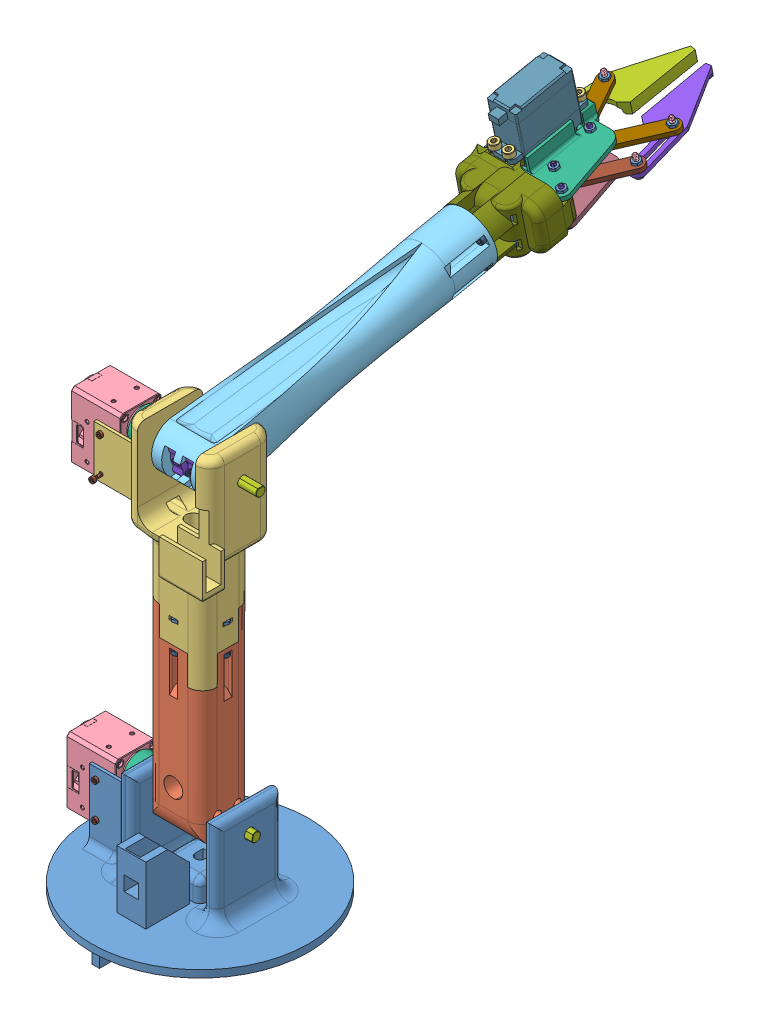
SolidWorks assembly Arm, configuration Défaut. Lengths in mm.
Overall size (155 388.61 426.09).
111 component instances, 29 part files, 108 mates.
Components (placement in the parent):
- arm_base-1: arm_base [Défaut] at (-76.3133 -23.0918 0) size (150 75 150)
- inferior_segment_1-1: inferior_segment_1 [Défaut] at (-77.3133 36.0082 -0.0041) x (1 0 0) z (0 0.001126 0.999999) size (42.86 137.5 35)
- superior_segment_1-1: superior_segment_1 [Défaut] at (-77.1133 116.0083 0.1059) x (1 0 0) z (0 0.001126 0.999999) size (91 145 55)
- XM430-W350-1: XM430-W350 [Default] at (-137.3133 32.4082 0) x (0 0 -1) z (1 0 0) size (28.5 46.5 42.4)
- segment_2-1: segment_2 [Default] at (-77.1133 240.5082 -0.0343) x (-1 0 0) z (0 0.200343 -0.979726) size (38.54 37.14 206.68)
- gripper-1: gripper [Predeterminado] at (-76.3096 293.9805 -248.1519) x (-1 0 0) z (0 -0.200343 0.979726) size (83.16 69.34 163.57)
  - superior_gripper_plate-1: superior_gripper_plate [Predeterminado] at (-28.7905 -8.0804 25) size (57.8 13.17 67.5)
  - left_gripper_tip-3: left_gripper_tip [Predeterminado] at (14.8599 7.4446 -59.2792) x (-0.991394 0 0.130911) z (0.130911 0 0.991394) size (24.38 8.18 79.76)
  - right_gripper_tip-3: right_gripper_tip [Predeterminado] at (-18.9029 4.2696 -55.4728) x (0.990618 0 0.13666) z (-0.13666 0 0.990618) size (24.38 8.18 79.76)
  - front_segment-1: front_segment [Predeterminado] at (10.4963 1.0946 -39.159) x (0.418148 0 -0.908379) z (0.908379 0 0.418148) size (49.52 3.17 9.53)
  - front_segment-2: front_segment [Predeterminado] at (-11.7671 1.0946 -38.0521) x (0.580265 0 0.814428) z (-0.814428 0 0.580265) size (49.52 3.17 9.53)
  - servo_gear_segment-1: servo_gear_segment [Predeterminado] at (23.393 1.0946 -5.3734) x (-0.403832 0 0.914833) z (-0.914833 0 -0.403832) size (56.02 3.17 23.48)
  - driven_gear_segment-1: driven_gear_segment [Predeterminado] at (-16.0335 1.0946 -8.1451) x (0.57026 0 0.821464) z (-0.821464 0 0.57026) size (56.51 3.17 22.67)
  - spacer-1: spacer [Predeterminado] at (-8.5405 -4.9054 11) x (0.999665 0 -0.025874) z (0.025874 0 0.999665) size (9.52 6 9.52)
  - spacer-2: spacer [Predeterminado] at (-8.5405 4.2696 11) x (0.999761 0 0.021872) z (-0.021872 0 0.999761) size (9.52 6 9.52)
  - spacer-4: spacer [Predeterminado] at (-4.0405 -4.9054 -19) x (0.999761 0 0.021872) z (-0.021872 0 0.999761) size (9.52 6 9.52)
  - spacer-5: spacer [Predeterminado] at (6.4595 4.2696 -19) x (0.999761 0 0.021872) z (-0.021872 0 0.999761) size (9.52 6 9.52)
  - spacer-6: spacer [Predeterminado] at (-4.0405 4.2696 -19) x (0.999761 0 0.021872) z (-0.021872 0 0.999761) size (9.52 6 9.52)
  - spacer-7: spacer [Predeterminado] at (6.4595 -4.9054 -19) x (0.228245 0 0.973604) z (-0.973604 0 0.228245) size (9.52 6 9.52)
  - inferior_gripper_plate-2: inferior_gripper_plate [Predeterminado] at (-28.7905 10.2696 25) size (57.8 3.17 62.5)
  - DS3218MG.stp-1: DS3218MG.stp [Défaut] at (20.9595 -47.3505 20.63) x (0 0 -1) z (1 0 0) size (54.67 45.39 20.26)
  - servo_motor_coupler-1: servo_motor_coupler [Défaut] at (10.9595 1.0946 11) x (-0.914833 0 -0.403832) z (-0.403832 0 0.914833) size (14.52 5.9 34.13)
  - spacer-8: spacer [Predeterminado] at (10.9595 4.2696 11) size (9.52 6 9.52)
  - gripper_arm_coupler-1: gripper_arm_coupler [Default] at (1.2085 2.6796 63) x (-1 0 0) z (0 0 -1) size (60.78 38.77 47.5)
  - M3-25mm_TYPE 18-8 SS SOCKET HEAD CAP SCREW-1: M3-25mm_TYPE 18-8 SS SOCKET HEAD CAP SCREW [91292A123] at (25.1104 -11.5554 20) x (-0.891625 0 -0.452774) z (0 -1 0) size (5.5 5.5 28.3)
  - M3-25mm_TYPE 18-8 SS SOCKET HEAD CAP SCREW-2: M3-25mm_TYPE 18-8 SS SOCKET HEAD CAP SCREW [91292A123] at (-22.6915 -11.5554 20) x (0.999554 0 -0.029869) z (0 -1 0) size (5.5 5.5 28.3)
  - M3-25mm_TYPE 18-8 SS SOCKET HEAD CAP SCREW-3: M3-25mm_TYPE 18-8 SS SOCKET HEAD CAP SCREW [91292A123] at (-4.0405 -11.5554 -19) x (0.859756 0 -0.510706) z (0 -1 0) size (5.5 5.5 28.3)
  - M3-25mm_TYPE 18-8 SS SOCKET HEAD CAP SCREW-4: M3-25mm_TYPE 18-8 SS SOCKET HEAD CAP SCREW [91292A123] at (6.4595 -11.5554 -19) x (0.999959 0 0.00908) z (0 -1 0) size (5.5 5.5 28.3)
  - M3-25mm_TYPE 18-8 SS SOCKET HEAD CAP SCREW-5: M3-25mm_TYPE 18-8 SS SOCKET HEAD CAP SCREW [91292A123] at (-8.5405 -11.5554 11) x (0.454151 0 0.890925) z (0 -1 0) size (5.5 5.5 28.3)
  - M3-16mm_91292A115_TYPE 18-8 SS SOCKET HEAD CAP SCREW-1: M3-16mm_91292A115_TYPE 18-8 SS SOCKET HEAD CAP SCREW [91292A115] at (10.9595 -2.5554 11) x (0.918772 0 -0.394789) z (0 -1 0) size (5.5 5.5 19.25)
  - M3-NUT_90710A030_TYPE 18-8 SS THIN HEX NUT - DIN 439B-1: M3-NUT_90710A030_TYPE 18-8 SS THIN HEX NUT - DIN 439B [90710A030] at (25.1104 -8.9804 20) x (-0.194301 0 0.980942) z (-0.980942 0 -0.194301) size (5.5 2.19 6.35)
  - M3-NUT_90710A030_TYPE 18-8 SS THIN HEX NUT - DIN 439B-2: M3-NUT_90710A030_TYPE 18-8 SS THIN HEX NUT - DIN 439B [90710A030] at (-8.5405 -8.9804 11) size (5.5 2.19 6.35)
  - M3-NUT_90710A030_TYPE 18-8 SS THIN HEX NUT - DIN 439B-3: M3-NUT_90710A030_TYPE 18-8 SS THIN HEX NUT - DIN 439B [90710A030] at (-4.0405 -8.9804 -19) size (5.5 2.19 6.35)
  - M3-NUT_90710A030_TYPE 18-8 SS THIN HEX NUT - DIN 439B-4: M3-NUT_90710A030_TYPE 18-8 SS THIN HEX NUT - DIN 439B [90710A030] at (-22.6915 -8.9804 20) size (5.5 2.19 6.35)
  - M3-NUT_90710A030_TYPE 18-8 SS THIN HEX NUT - DIN 439B-5: M3-NUT_90710A030_TYPE 18-8 SS THIN HEX NUT - DIN 439B [90710A030] at (6.4595 -7.8304 -19) size (5.5 2.19 6.35)
  - M4-NUT_90710A035_TYPE 18-8 SS THIN HEX NUT - DIN 439B-1: M4-NUT_90710A035_TYPE 18-8 SS THIN HEX NUT - DIN 439B [90710A035] at (5.9595 -10.9804 -24.15) x (0.99976 0 -0.021901) z (0.021901 0 0.99976) size (7 2.75 8.08)
  - M4-NUT_90710A035_TYPE 18-8 SS THIN HEX NUT - DIN 439B-2: M4-NUT_90710A035_TYPE 18-8 SS THIN HEX NUT - DIN 439B [90710A035] at (15.9595 -10.9804 -24.15) size (7 2.75 8.08)
  - M4-12mm_TYPE 18-8 SS SOCKET HEAD CAP SCREW-1: M4-12mm_TYPE 18-8 SS SOCKET HEAD CAP SCREW [91292A118] at (5.9595 -7.6505 25.35) x (0.655946 0 0.754807) z (0 1 0) size (7 7 16.33)
  - M4-12mm_TYPE 18-8 SS SOCKET HEAD CAP SCREW-2: M4-12mm_TYPE 18-8 SS SOCKET HEAD CAP SCREW [91292A118] at (15.9595 -7.6505 25.35) x (0.901182 0 0.43344) z (0 1 0) size (7 7 16.33)
  - M4-NUT_90710A035_TYPE 18-8 SS THIN HEX NUT - DIN 439B-3: M4-NUT_90710A035_TYPE 18-8 SS THIN HEX NUT - DIN 439B [90710A035] at (15.9595 -11.0704 25.35) x (0.993077 0 0.117463) z (-0.117463 0 0.993077) size (7 2.75 8.08)
  - M4-NUT_90710A035_TYPE 18-8 SS THIN HEX NUT - DIN 439B-4: M4-NUT_90710A035_TYPE 18-8 SS THIN HEX NUT - DIN 439B [90710A035] at (5.9595 -11.0704 25.35) x (-0.238209 0 0.971214) z (-0.971214 0 -0.238209) size (7 2.75 8.08)
  - M3-12mm_91292A114_TYPE 18-8 SS SOCKET HEAD CAP SCREW-1: M3-12mm_91292A114_TYPE 18-8 SS SOCKET HEAD CAP SCREW [91292A114] at (-27.2511 -4.5554 -51.5771) x (0.831997 0 -0.55478) z (0 -1 0) size (5.5 5.5 15.23)
  - M3-12mm_91292A114_TYPE 18-8 SS SOCKET HEAD CAP SCREW-2: M3-12mm_91292A114_TYPE 18-8 SS SOCKET HEAD CAP SCREW [91292A114] at (-31.3509 -4.5554 -21.8586) x (-0.907237 0 -0.42062) z (0 -1 0) size (5.5 5.5 15.23)
  - M3-12mm_91292A114_TYPE 18-8 SS SOCKET HEAD CAP SCREW-3: M3-12mm_91292A114_TYPE 18-8 SS SOCKET HEAD CAP SCREW [91292A114] at (23.1854 -4.5554 -55.3352) x (-0.45795 0 -0.888978) z (0 -1 0) size (5.5 5.5 15.23)
  - M3-12mm_91292A114_TYPE 18-8 SS SOCKET HEAD CAP SCREW-4: M3-12mm_91292A114_TYPE 18-8 SS SOCKET HEAD CAP SCREW [91292A114] at (27.1127 -4.5554 -25.5933) x (-0.617984 0 -0.786191) z (0 -1 0) size (5.5 5.5 15.23)
  - M3-NUT_90710A030_TYPE 18-8 SS THIN HEX NUT - DIN 439B-7: M3-NUT_90710A030_TYPE 18-8 SS THIN HEX NUT - DIN 439B [90710A030] at (27.1127 0.1946 -25.5933) x (0.973179 0 0.23005) z (-0.23005 0 0.973179) size (5.5 2.19 6.35)
  - M3-NUT_90710A030_TYPE 18-8 SS THIN HEX NUT - DIN 439B-8: M3-NUT_90710A030_TYPE 18-8 SS THIN HEX NUT - DIN 439B [90710A030] at (23.1854 0.1946 -55.3352) x (0.934993 0 0.354665) z (-0.354665 0 0.934993) size (5.5 2.19 6.35)
  - M3-NUT_90710A030_TYPE 18-8 SS THIN HEX NUT - DIN 439B-9: M3-NUT_90710A030_TYPE 18-8 SS THIN HEX NUT - DIN 439B [90710A030] at (-31.3509 0.1946 -21.8586) x (0.443225 0 -0.89641) z (0.89641 0 0.443225) size (5.5 2.19 6.35)
  - M3-NUT_90710A030_TYPE 18-8 SS THIN HEX NUT - DIN 439B-10: M3-NUT_90710A030_TYPE 18-8 SS THIN HEX NUT - DIN 439B [90710A030] at (-27.2511 0.1946 -51.5771) x (0.696424 0 -0.717631) z (0.717631 0 0.696424) size (5.5 2.19 6.35)
  - M4-12mm_TYPE 18-8 SS SOCKET HEAD CAP SCREW-3: M4-12mm_TYPE 18-8 SS SOCKET HEAD CAP SCREW [91292A118] at (15.9595 -7.6505 -24.15) x (0.999512 0 -0.031235) z (0 1 0) size (7 7 16.33)
  - M4-12mm_TYPE 18-8 SS SOCKET HEAD CAP SCREW-4: M4-12mm_TYPE 18-8 SS SOCKET HEAD CAP SCREW [91292A118] at (5.9595 -7.6505 -24.15) x (0.998964 0 -0.045509) z (0 1 0) size (7 7 16.33)
  - M3-8mm_91292A112_TYPE 18-8 SS SOCKET HEAD CAP SCREW-3: M3-8mm_91292A112_TYPE 18-8 SS SOCKET HEAD CAP SCREW [91292A112] at (20.6595 -3.7304 -10.9743) x (0.858818 0 -0.512282) z (0 -1 0) size (5.5 5.5 11.2)
- XM430-W350-2: XM430-W350 [Default] at (-134.1133 240.5082 -0.0343) x (0 -0.001126 -0.999999) z (1 0 0) size (28.5 46.5 42.4)
- Coupler_Joint3-3: Coupler_Joint3 [Défaut] at (-115.3133 32.4082 0) x (0 -0.685146 0.728406) z (0 0.728406 0.685146) size (22.5 11 20.75)
- Coupler_Joint3-4: Coupler_Joint3 [Défaut] at (-112.1133 240.5082 -0.0343) x (0 -0.431326 0.902196) z (0 0.902196 0.431326) size (22.5 11 20.75)
- shaft-1: shaft [3po] at (-75.8133 32.4082 0) x (0 0.977649 -0.210244) z (1 0 0) size (6.35 5.71 76.2)
- 545548_hub-1: 545548_hub [Default] at (-89.3797 41.3353 -38.9212) x (0 -0.001126 -0.999999) z (0 -0.999999 0.001126) size (20.57 9.53 20.57)
  - 545548 assembly.STEP-1: 545548 assembly.STEP [Default] at origin size (20.57 9.53 20.57)
    - 545548.STEP-1: 545548.STEP [Default] at (-38.9112 12.0765 8.9709) size (20.57 9.53 20.57)
    - 632138_91375A438.STEP-1: 632138_91375A438.STEP [Default] at (-38.9112 18.109 15.0823) x (0.93363 0.358238 0) z (0 0 1) size (4.83 4.83 6.36)
- 545548_hub-2: 545548_hub [Default] at (-65.2468 41.4229 38.901) x (0 0.001126 0.999999) z (0 -0.999999 0.001126) size (20.57 9.53 20.57)
  - 545548 assembly.STEP-1: 545548 assembly.STEP [Default] at origin size (20.57 9.53 20.57)
    - 545548.STEP-1: 545548.STEP [Default] at (-38.9112 12.0765 8.9709) size (20.57 9.53 20.57)
    - 632138_91375A438.STEP-1: 632138_91375A438.STEP [Default] at (-38.9112 18.109 15.0823) x (0.93363 0.358238 0) z (0 0 1) size (4.83 4.83 6.36)
- 545548_hub-3: 545548_hub [Default] at (-65.0368 280.4338 -0.7485) x (0 0.9783 0.207191) z (0 -0.207191 0.9783) size (20.57 9.53 20.57)
  - 545548 assembly.STEP-1: 545548 assembly.STEP [Default] at origin size (20.57 9.53 20.57)
    - 545548.STEP-1: 545548.STEP [Default] at (-38.9112 12.0765 8.9709) size (20.57 9.53 20.57)
    - 632138_91375A438.STEP-1: 632138_91375A438.STEP [Default] at (-38.9112 18.109 15.0823) x (0.93363 0.358238 0) z (0 0 1) size (4.83 4.83 6.36)
- 545548_hub-4: 545548_hub [Default] at (-89.1897 204.1832 -16.619) x (0 -0.979726 -0.200343) z (0 -0.200343 0.979726) size (20.57 9.53 20.57)
  - 545548 assembly.STEP-1: 545548 assembly.STEP [Default] at origin size (20.57 9.53 20.57)
    - 545548.STEP-1: 545548.STEP [Default] at (-38.9112 12.0765 8.9709) size (20.57 9.53 20.57)
    - 632138_91375A438.STEP-1: 632138_91375A438.STEP [Default] at (-38.9112 18.109 15.0823) x (0.93363 0.358238 0) z (0 0 1) size (4.83 4.83 6.36)
- shaft-2: shaft [3po] at (-72.6133 240.5082 -0.0343) x (0 0 1) z (-1 0 0) size (6.35 5.71 76.2)
- M3-20mm_91292A123_TYPE 18-8 SS SOCKET HEAD CAP SCREW-1: M3-20mm_91292A123_TYPE 18-8 SS SOCKET HEAD CAP SCREW [91292A123] at (-92.7783 39.3307 6.907) x (0 -0.587196 0.809445) z (-1 0 0) size (5.5 5.5 28.3)
- M3-20mm_91292A123_TYPE 18-8 SS SOCKET HEAD CAP SCREW-2: M3-20mm_91292A123_TYPE 18-8 SS SOCKET HEAD CAP SCREW [91292A123] at (-92.7783 25.4854 -6.9072) x (0 -0.208065 0.978115) z (-1 0 0) size (5.5 5.5 28.3)
- M3-20mm_91292A123_TYPE 18-8 SS SOCKET HEAD CAP SCREW-3: M3-20mm_91292A123_TYPE 18-8 SS SOCKET HEAD CAP SCREW [91292A123] at (-61.8483 39.3154 -6.9228) x (0 0.935615 -0.353022) z (1 0 0) size (5.5 5.5 28.3)
- M3-20mm_91292A123_TYPE 18-8 SS SOCKET HEAD CAP SCREW-4: M3-20mm_91292A123_TYPE 18-8 SS SOCKET HEAD CAP SCREW [91292A123] at (-61.8483 25.5009 6.9228) x (0 0.227771 -0.973715) z (1 0 0) size (5.5 5.5 28.3)
- M3-20mm_91292A123_TYPE 18-8 SS SOCKET HEAD CAP SCREW-5: M3-20mm_91292A123_TYPE 18-8 SS SOCKET HEAD CAP SCREW [91292A123] at (-92.5883 232.3483 5.3549) x (0 -0.37577 0.926713) z (-1 0 0) size (5.5 5.5 28.3)
- M3-20mm_91292A123_TYPE 18-8 SS SOCKET HEAD CAP SCREW-6: M3-20mm_91292A123_TYPE 18-8 SS SOCKET HEAD CAP SCREW [91292A123] at (-92.5883 248.6682 -5.4236) x (0 -0.381897 0.924205) z (-1 0 0) size (5.5 5.5 28.3)
- M3-20mm_91292A123_TYPE 18-8 SS SOCKET HEAD CAP SCREW-7: M3-20mm_91292A123_TYPE 18-8 SS SOCKET HEAD CAP SCREW [91292A123] at (-61.6383 235.062 -8.1564) x (0 0.397711 -0.917511) z (1 0 0) size (5.5 5.5 28.3)
- M3-20mm_91292A123_TYPE 18-8 SS SOCKET HEAD CAP SCREW-8: M3-20mm_91292A123_TYPE 18-8 SS SOCKET HEAD CAP SCREW [91292A123] at (-61.6383 245.8975 8.1256) x (0 -0.001632 -0.999999) z (1 0 0) size (5.5 5.5 28.3)
- M3-20mm_91292A123_TYPE 18-8 SS SOCKET HEAD CAP SCREW-9: M3-20mm_91292A123_TYPE 18-8 SS SOCKET HEAD CAP SCREW [91292A123] at (-63.6133 291.4688 -206.8171) x (-0.995353 -0.09434 -0.019291) z (0 0.200343 -0.979726) size (5.5 5.5 28.3)
- M3-20mm_91292A123_TYPE 18-8 SS SOCKET HEAD CAP SCREW-10: M3-20mm_91292A123_TYPE 18-8 SS SOCKET HEAD CAP SCREW [91292A123] at (-63.6133 274.8135 -210.2229) x (-0.985953 -0.163635 -0.033462) z (0 0.200343 -0.979726) size (5.5 5.5 28.3)
- M3-20mm_91292A123_TYPE 18-8 SS SOCKET HEAD CAP SCREW-11: M3-20mm_91292A123_TYPE 18-8 SS SOCKET HEAD CAP SCREW [91292A123] at (-90.6133 291.4688 -206.8171) x (-0.201765 0.959577 0.196222) z (0 0.200343 -0.979726) size (5.5 5.5 28.3)
- M3-20mm_91292A123_TYPE 18-8 SS SOCKET HEAD CAP SCREW-12: M3-20mm_91292A123_TYPE 18-8 SS SOCKET HEAD CAP SCREW [91292A123] at (-90.6133 274.8135 -210.2229) x (-0.924082 0.374446 0.07657) z (0 0.200343 -0.979726) size (5.5 5.5 28.3)
- M3-NUT_90710A030_TYPE 18-8 SS THIN HEX NUT - DIN 439B-1: M3-NUT_90710A030_TYPE 18-8 SS THIN HEX NUT - DIN 439B [90710A030] at (-90.6133 273.391 -203.2669) x (-0.664039 0.732539 0.149796) z (-0.747698 -0.650577 -0.133035) size (5.5 2.19 6.35)
- M3-NUT_90710A030_TYPE 18-8 SS THIN HEX NUT - DIN 439B-2: M3-NUT_90710A030_TYPE 18-8 SS THIN HEX NUT - DIN 439B [90710A030] at (-63.6133 273.391 -203.2669) x (0.753429 0.644198 0.131731) z (-0.657529 0.738154 0.150944) size (5.5 2.19 6.35)
- M3-NUT_90710A030_TYPE 18-8 SS THIN HEX NUT - DIN 439B-3: M3-NUT_90710A030_TYPE 18-8 SS THIN HEX NUT - DIN 439B [90710A030] at (-63.6133 290.0464 -199.861) x (0.94811 0.311495 0.063697) z (-0.317941 0.928888 0.189947) size (5.5 2.19 6.35)
- M3-NUT_90710A030_TYPE 18-8 SS THIN HEX NUT - DIN 439B-4: M3-NUT_90710A030_TYPE 18-8 SS THIN HEX NUT - DIN 439B [90710A030] at (-90.6133 290.0464 -199.861) x (0.320226 -0.928135 -0.189793) z (0.947341 0.313733 0.064155) size (5.5 2.19 6.35)
- M3-20mm_91292A123_TYPE 18-8 SS SOCKET HEAD CAP SCREW-13: M3-20mm_91292A123_TYPE 18-8 SS SOCKET HEAD CAP SCREW [91292A123] at (-77.3133 158.0253 15.1586) x (0.920814 0.000439 0.390003) z (0 0.999999 -0.001126) size (5.5 5.5 28.3)
- M3-20mm_91292A123_TYPE 18-8 SS SOCKET HEAD CAP SCREW-14: M3-20mm_91292A123_TYPE 18-8 SS SOCKET HEAD CAP SCREW [91292A123] at (-59.5133 158.0081 -0.1414) x (0.792253 -0.000687 -0.610192) z (0 0.999999 -0.001126) size (5.5 5.5 28.3)
- M3-20mm_91292A123_TYPE 18-8 SS SOCKET HEAD CAP SCREW-15: M3-20mm_91292A123_TYPE 18-8 SS SOCKET HEAD CAP SCREW [91292A123] at (-77.3133 157.9908 -15.4414) x (0.147292 -0.001114 -0.989092) z (0 0.999999 -0.001126) size (5.5 5.5 28.3)
- M3-20mm_91292A123_TYPE 18-8 SS SOCKET HEAD CAP SCREW-16: M3-20mm_91292A123_TYPE 18-8 SS SOCKET HEAD CAP SCREW [91292A123] at (-95.1133 158.0081 -0.1414) x (-0.185479 -0.001107 -0.982648) z (0 0.999999 -0.001126) size (5.5 5.5 28.3)
- M3-NUT_90710A030_TYPE 18-8 SS THIN HEX NUT - DIN 439B-5: M3-NUT_90710A030_TYPE 18-8 SS THIN HEX NUT - DIN 439B [90710A030] at (-77.3133 150.9253 15.1666) x (0.62194 -0.000882 -0.783065) z (0.783065 0.0007 0.621939) size (5.5 2.19 6.35)
- M3-NUT_90710A030_TYPE 18-8 SS THIN HEX NUT - DIN 439B-6: M3-NUT_90710A030_TYPE 18-8 SS THIN HEX NUT - DIN 439B [90710A030] at (-77.3133 150.8908 -15.4334) x (0.954232 0.000337 0.299066) z (-0.299067 0.001075 0.954232) size (5.5 2.19 6.35)
- M3-NUT_90710A030_TYPE 18-8 SS THIN HEX NUT - DIN 439B-7: M3-NUT_90710A030_TYPE 18-8 SS THIN HEX NUT - DIN 439B [90710A030] at (-95.1133 150.9081 -0.1334) x (0.978558 0.000232 0.20597) z (-0.205971 0.001102 0.978558) size (5.5 2.19 6.35)
- M3-NUT_90710A030_TYPE 18-8 SS THIN HEX NUT - DIN 439B-8: M3-NUT_90710A030_TYPE 18-8 SS THIN HEX NUT - DIN 439B [90710A030] at (-59.5133 150.9081 -0.1334) x (0.816024 -0.000651 -0.578017) z (0.578018 0.000919 0.816024) size (5.5 2.19 6.35)
- M2-8mm_91292A832_TYPE 18-8 SS SOCKET HEAD CAP SCREW-1: M2-8mm_91292A832_TYPE 18-8 SS SOCKET HEAD CAP SCREW [91292A832] at (-128.1133 236.4987 -8.5298) x (1 0 0) z (0 0.001126 0.999999) size (3.8 3.8 10.11)
- M2-8mm_91292A832_TYPE 18-8 SS SOCKET HEAD CAP SCREW-2: M2-8mm_91292A832_TYPE 18-8 SS SOCKET HEAD CAP SCREW [91292A832] at (-128.1133 212.4987 -8.5028) x (1 0 0) z (0 0.001126 0.999999) size (3.8 3.8 10.11)
- M2-8mm_91292A832_TYPE 18-8 SS SOCKET HEAD CAP SCREW-3: M2-8mm_91292A832_TYPE 18-8 SS SOCKET HEAD CAP SCREW [91292A832] at (-128.1133 236.5178 8.4702) x (1 0 0) z (0 -0.001126 -0.999999) size (3.8 3.8 10.11)
- M2-8mm_91292A832_TYPE 18-8 SS SOCKET HEAD CAP SCREW-4: M2-8mm_91292A832_TYPE 18-8 SS SOCKET HEAD CAP SCREW [91292A832] at (-128.1133 212.2222 13.4376) x (1 0 0) z (0 0.026321 -0.999654) size (3.8 3.8 10.11)
- M2-8mm_91292A832_TYPE 18-8 SS SOCKET HEAD CAP SCREW-5: M2-8mm_91292A832_TYPE 18-8 SS SOCKET HEAD CAP SCREW [91292A832] at (-131.3133 28.4082 -8.5) x (0.974899 -0.222647 0) z (0 0 1) size (3.8 3.8 10.11)
- M2-8mm_91292A832_TYPE 18-8 SS SOCKET HEAD CAP SCREW-6: M2-8mm_91292A832_TYPE 18-8 SS SOCKET HEAD CAP SCREW [91292A832] at (-131.3133 4.4082 -8.5) size (3.8 3.8 10.11)
- M2-8mm_91292A832_TYPE 18-8 SS SOCKET HEAD CAP SCREW-7: M2-8mm_91292A832_TYPE 18-8 SS SOCKET HEAD CAP SCREW [91292A832] at (-131.3133 28.4082 8.5) x (0.974899 -0.222647 0) z (0 0 -1) size (3.8 3.8 10.11)
- M2-8mm_91292A832_TYPE 18-8 SS SOCKET HEAD CAP SCREW-8: M2-8mm_91292A832_TYPE 18-8 SS SOCKET HEAD CAP SCREW [91292A832] at (-131.3133 4.4082 8.5) x (1 0 0) z (0 0 -1) size (3.8 3.8 10.11)
- M2-8mm_91292A832_TYPE 18-8 SS SOCKET HEAD CAP SCREW-9: M2-8mm_91292A832_TYPE 18-8 SS SOCKET HEAD CAP SCREW [91292A832] at (-120.6133 37.8893 -5.8272) x (0 -0.284236 0.958754) z (-1 0 0) size (3.8 3.8 10.11)
- M2-8mm_91292A832_TYPE 18-8 SS SOCKET HEAD CAP SCREW-10: M2-8mm_91292A832_TYPE 18-8 SS SOCKET HEAD CAP SCREW [91292A832] at (-120.6133 38.2354 5.4812) x (0 -0.570348 0.821403) z (-1 0 0) size (3.8 3.8 10.11)
- M2-8mm_91292A832_TYPE 18-8 SS SOCKET HEAD CAP SCREW-11: M2-8mm_91292A832_TYPE 18-8 SS SOCKET HEAD CAP SCREW [91292A832] at (-120.6133 26.927 5.8272) x (0 0.623735 0.781636) z (-1 0 0) size (3.8 3.8 10.11)
- M2-8mm_91292A832_TYPE 18-8 SS SOCKET HEAD CAP SCREW-12: M2-8mm_91292A832_TYPE 18-8 SS SOCKET HEAD CAP SCREW [91292A832] at (-117.4133 243.9589 -7.2519) x (0 -0.229339 0.973347) z (-1 0 0) size (3.8 3.8 10.11)
- M2-8mm_91292A832_TYPE 18-8 SS SOCKET HEAD CAP SCREW-13: M2-8mm_91292A832_TYPE 18-8 SS SOCKET HEAD CAP SCREW [91292A832] at (-117.4133 247.7258 3.4163) x (0 -0.222004 0.975046) z (-1 0 0) size (3.8 3.8 10.11)
- M2-8mm_91292A832_TYPE 18-8 SS SOCKET HEAD CAP SCREW-14: M2-8mm_91292A832_TYPE 18-8 SS SOCKET HEAD CAP SCREW [91292A832] at (-117.4133 237.0576 7.1832) x (0 -0.647559 0.762015) z (-1 0 0) size (3.8 3.8 10.11)
Mates (geometry in assembly coordinates):
- Coaxiale1: concentric anti-aligned: circle of BArm-1; circle of VArm1_bolt-1
- Distance1: distance = 3 mm anti-aligned: plane of VArm1_bolt-1 through (-97.3133 156.0278 17.3608) normal (-1 0 0); plane of BArm-1 through (-100.3133 46.9082 -75) normal (1 0 0)
- Coïncidente3: coincident anti-aligned: plane of inferior_segment_1-1 through (-77.3133 116.0081 -0.0941) normal (0 0.999999 -0.001126); plane of superior_segment_1-1 through (-77.1133 116.0083 0.1059) normal (0 -0.999999 0.001126)
- Distance3: distance = 0.2 mm anti-aligned: plane of superior_segment_1-1 through (-67.3133 136.028 17.5833) normal (-1 0 0); plane of inferior_segment_1-1 through (-67.5133 116.0278 17.4059) normal (1 0 0)
- Distance4: distance = 0.2 mm anti-aligned: plane of superior_segment_1-1 through (-67.3133 136.0165 7.3833) normal (0 -0.001126 -0.999999); plane of inferior_segment_1-1 through (-57.3133 116.0163 7.2059) normal (0 0.001126 0.999999)
- Coaxiale3: concentric aligned: cylinder of BArm-1 through (-103.3133 32.4082 0) axis (1 0 0) radius 6.55; cylinder of XM430-W350-1 through (-116.4133 32.4082 0) axis (1 0 0) radius 2.25
- Parallèle1: parallel aligned: plane of BArm-1 through (-136.3133 -13.0918 -16.5) normal (0 0 -1); plane of XM430-W350-1 through (-154.3133 -2.8418 -14.25) normal (0 0 -1)
- Largeur1: width aligned: plane of XM430-W350-1 through (-154.3133 -2.8418 -14.25) normal (0 0 -1); plane of XM430-W350-1 through (-154.3133 43.6582 14.25) normal (0 0 1); plane of BArm-1 through (-105.5633 44.9082 14.5) normal (0 0 -1); plane of BArm-1 through (-105.5633 44.9082 -14.5) normal (0 0 1)
- Coaxiale4: concentric aligned: cylinder of superior_segment_1-1 through (-47.1133 240.5082 -0.0343) axis (-1 0 0) radius 3.35; cylinder of Segment_2-1/Bras_Horizontal-1 through (-97.3643 239.9956 14.5982) axis (-1 0 0) radius 3.3734
- Coaxiale6: concentric anti-aligned: cylinder of BArm-1 through (-76.3133 -28.0918 0) axis (0 1 0) radius 50.55; cylinder of Support_Bearing_V4-1 through (-76.3133 -138.2606 0) axis (0 -1 0) radius 50
- Coaxiale9: concentric anti-aligned: cylinder of superior_segment_1-1 through (-47.1133 240.5082 -0.0343) axis (-1 0 0) radius 3.35; cylinder of segment_2-1 through (-57.1472 240.5082 -0.0343) axis (1 0 0) radius 3.3734
- Coïncidente4: coincident anti-aligned: plane of Bras_Horizontal-1 through (-77.1133 278.7336 -186.966) normal (0 0.200343 -0.979726); plane of Gripper-1/gripper_arm_coupler-1 through (-77.5181 278.7336 -186.966) normal (0 -0.200343 0.979726)
- Coaxiale10: concentric anti-aligned: cylinder of Bras_Horizontal-1 through (-90.6133 270.4059 -188.6689) axis (0 0.200343 -0.979726) radius 1.7; cylinder of Gripper-1/gripper_arm_coupler-1 through (-90.6133 270.4059 -188.6689) axis (0 -0.200343 0.979726) radius 1.7
- Parallèle2: parallel aligned: plane of Bras_Horizontal-1 through (-57.842 283.766 -182.8749) normal (0 0.979726 0.200343); plane of Gripper-1/gripper_arm_coupler-1 through (-68.0181 283.8772 -185.9142) normal (0 0.979726 0.200343)
- Largeur2: width aligned: plane of segment_2-1 through (-94.0793 240.5082 -0.0343) normal (-1 0 0); plane of segment_2-1 through (-60.1472 240.5082 -0.0343) normal (1 0 0); plane of superior_segment_1-1 through (-57.1133 260.9829 -22.5574) normal (-1 0 0); plane of superior_segment_1-1 through (-97.1133 260.9829 -22.5574) normal (1 0 0)
- Largeur3: width aligned: plane of XM430-W350-2 through (-151.1133 251.7743 14.203) normal (0 0.001126 0.999999); plane of XM430-W350-2 through (-151.1133 205.2422 -14.2446) normal (0 -0.001126 -0.999999); plane of superior_segment_1-1 through (-102.3633 253.9919 -14.5495) normal (0 0.001126 0.999999); plane of superior_segment_1-1 through (-102.3633 254.0246 14.4505) normal (0 -0.001126 -0.999999)
- Parallèle3: parallel aligned: plane of superior_segment_1-1 through (-102.1133 241.5268 16.4645) normal (0 0.999999 -0.001126); plane of XM430-W350-2 through (-151.1133 251.7422 -14.297) normal (0 0.999999 -0.001126)
- Coaxiale11: concentric anti-aligned: cylinder of superior_segment_1-1 through (-47.1133 240.5082 -0.0343) axis (-1 0 0) radius 3.35; cylinder of XM430-W350-2 through (-113.2133 240.5082 -0.0343) axis (1 0 0) radius 2.25
- Coïncidente6: coincident anti-aligned: plane of XM430-W350-1 through (-118.3133 32.4082 0) normal (1 0 0); plane of Coupler_Joint3-3 through (-118.3133 32.4082 0) normal (-1 0 0)
- Coaxiale12: concentric anti-aligned: cylinder of XM430-W350-1 through (-116.4133 32.4082 0) axis (1 0 0) radius 2.25; cylinder of Coupler_Joint3-3 through (-116.3133 32.4082 0) axis (-1 0 0) radius 4.25
- Coïncidente8: coincident anti-aligned: plane of XM430-W350-2 through (-115.1133 240.5082 -0.0343) normal (1 0 0); plane of coupler_joint3-4 through (-115.1133 240.5082 -0.0343) normal (-1 0 0)
- Coaxiale13: concentric anti-aligned: cylinder of XM430-W350-2 through (-113.2133 240.5082 -0.0343) axis (1 0 0) radius 2.25; cylinder of coupler_joint3-4 through (-113.1133 240.5082 -0.0343) axis (-1 0 0) radius 4.25
- Coaxiale14: concentric anti-aligned: cylinder of superior_segment_1-1 through (-128.1133 236.4829 -22.5298) axis (0 0.001126 0.999999) radius 1.35; cylinder of XM430-W350-2 through (-128.1133 236.52 10.4235) axis (0 -0.001126 -0.999999) radius 1.025
- Coaxiale15: concentric aligned: cylinder of BArm-1 through (-131.3133 28.4082 75) axis (0 0 -1) radius 1.35; cylinder of XM430-W350-1 through (-131.3133 28.4082 10.4533) axis (0 0 -1) radius 1.025
- Coïncidente10: coincident anti-aligned: plane of XM430-W350-1 through (-113.9133 32.4082 0) normal (1 0 0); plane of shaft-1 through (-113.9133 32.4082 0) normal (-1 0 0)
- Coaxiale16: concentric anti-aligned: cone of XM430-W350-1 through (-113.9883 32.4082 0) axis (1 0 0); cylinder of shaft-1 through (-37.7133 32.4082 0) axis (-1 0 0) radius 3.175
- Coaxiale17: concentric anti-aligned: cylinder of shaft-1 through (-37.7133 32.4082 0) axis (-1 0 0) radius 3.175; cylinder of 545548_hub-1/545548 assembly.STEP-1/545548.STEP-1 through (-67.7783 32.4082 0) axis (1 0 0) radius 3.175
- Coaxiale18: concentric aligned: cylinder of VArm1_bolt-1 through (-57.3133 25.5009 6.9228) axis (1 0 0) radius 2.65; cone of 545548_hub-1/545548 assembly.STEP-1/545548.STEP-1 through (-74.7633 25.5011 6.9226) axis (1 0 0)
- Coaxiale19: concentric aligned: cylinder of shaft-1 through (-37.7133 32.4082 0) axis (-1 0 0) radius 3.175; cylinder of 545548_hub-2/545548 assembly.STEP-1/545548.STEP-1 through (-86.8483 32.4082 0) axis (-1 0 0) radius 3.175
- Coaxiale20: concentric aligned: cylinder of VArm1_bolt-1 through (-97.3133 25.5009 6.9228) axis (-1 0 0) radius 2.75; cone of 545548_hub-2/545548 assembly.STEP-1/545548.STEP-1 through (-79.8633 25.5011 6.9226) axis (-1 0 0)
- Coaxiale21: concentric anti-aligned: cylinder of Bras_Horizontal-1 through (-57.1472 240.5082 -0.0343) axis (1 0 0) radius 3.3734; cylinder of 545548_hub-3/545548 assembly.STEP-1/545548.STEP-1 through (-86.6383 240.5082 -0.0343) axis (-1 0 0) radius 3.175
- Coaxiale22: concentric aligned: cylinder of Bras_Horizontal-1 through (-97.0793 232.3108 5.2977) axis (-1 0 0) radius 2.75; cone of 545548_hub-3/545548 assembly.STEP-1/545548.STEP-1 through (-79.6533 232.3108 5.2977) axis (-1 0 0)
- Coaxiale23: concentric aligned: cylinder of Bras_Horizontal-1 through (-57.1472 240.5082 -0.0343) axis (1 0 0) radius 3.3734; cylinder of 545548_hub-4/545548 assembly.STEP-1/545548.STEP-1 through (-67.5883 240.5082 -0.0343) axis (1 0 0) radius 3.175
- Coaxiale24: concentric aligned: cylinder of Bras_Horizontal-1 through (-57.1472 232.3483 5.3549) axis (1 0 0) radius 2.75; cone of 545548_hub-4/545548 assembly.STEP-1/545548.STEP-1 through (-74.5733 232.3483 5.3549) axis (1 0 0)
- Coïncidente15: coincident anti-aligned: plane of Bras_Horizontal-1 through (-74.5733 249.0793 7.264) normal (1 0 0); plane of 545548_hub-4/545548 assembly.STEP-1/545548.STEP-1 through (-74.5733 244.5882 -2.729) normal (-1 0 0)
- Coïncidente16: coincident anti-aligned: plane of Bras_Horizontal-1 through (-79.6533 249.0793 7.264) normal (-1 0 0); plane of 545548_hub-3/545548 assembly.STEP-1/545548.STEP-1 through (-79.6533 237.8422 -4.133) normal (1 0 0)
- Coïncidente17: coincident anti-aligned: plane of XM430-W350-2 through (-110.7133 240.5082 -0.0343) normal (1 0 0); plane of shaft-2 through (-110.7133 240.5082 -0.0343) normal (-1 0 0)
- Coaxiale25: concentric aligned: cone of XM430-W350-2 through (-110.7883 240.5082 -0.0343) axis (1 0 0); cylinder of shaft-2 through (-110.7133 240.5082 -0.0343) axis (1 0 0) radius 3.175
- Coïncidente18: coincident anti-aligned: plane of VArm1_bolt-1 through (-74.7633 42.82 10.5383) normal (1 0 0); plane of 545548_hub-1/545548 assembly.STEP-1/545548.STEP-1 through (-74.7633 35.8694 3.4535) normal (-1 0 0)
- Coïncidente19: coincident anti-aligned: plane of VArm1_bolt-1 through (-79.8633 42.82 10.5383) normal (-1 0 0); plane of 545548_hub-2/545548 assembly.STEP-1/545548.STEP-1 through (-79.8633 35.8617 -3.4613) normal (1 0 0)
- Coïncidente20: coincident anti-aligned: plane of 545548_hub-1/545548 assembly.STEP-1/545548.STEP-1 through (-67.7783 35.8694 3.4535) normal (1 0 0); plane of M3-20mm_91292A123_TYPE 18-8 SS SOCKET HEAD CAP SCREW-1 through (-67.7783 39.3307 6.907) normal (-1 0 0)
- Coaxiale26: concentric aligned: cone of 545548_hub-1/545548 assembly.STEP-1/545548.STEP-1 through (-68.1783 39.3307 6.907) axis (-1 0 0); cylinder of M3-20mm_91292A123_TYPE 18-8 SS SOCKET HEAD CAP SCREW-1 through (-64.7783 39.3307 6.907) axis (-1 0 0) radius 2.75
- Coaxiale27: concentric anti-aligned: cylinder of inferior_segment_1-1 through (-57.3133 25.4854 -6.9072) axis (1 0 0) radius 2.65; cylinder of M3-20mm_91292A123_TYPE 18-8 SS SOCKET HEAD CAP SCREW-2 through (-64.7783 25.4854 -6.9072) axis (-1 0 0) radius 2.75
- Coïncidente21: coincident anti-aligned: plane of 545548_hub-1/545548 assembly.STEP-1/545548.STEP-1 through (-67.7783 35.8694 3.4535) normal (1 0 0); plane of M3-20mm_91292A123_TYPE 18-8 SS SOCKET HEAD CAP SCREW-2 through (-67.7783 25.4854 -6.9072) normal (-1 0 0)
- Coaxiale28: concentric anti-aligned: cylinder of inferior_segment_1-1 through (-97.3133 39.3154 -6.9228) axis (-1 0 0) radius 2.75; cylinder of M3-20mm_91292A123_TYPE 18-8 SS SOCKET HEAD CAP SCREW-3 through (-89.8483 39.3154 -6.9228) axis (1 0 0) radius 2.75
- Coïncidente22: coincident anti-aligned: plane of 545548_hub-2/545548 assembly.STEP-1/545548.STEP-1 through (-86.8483 35.8617 -3.4613) normal (-1 0 0); plane of M3-20mm_91292A123_TYPE 18-8 SS SOCKET HEAD CAP SCREW-3 through (-86.8483 39.3154 -6.9228) normal (1 0 0)
- Coaxiale29: concentric anti-aligned: cylinder of inferior_segment_1-1 through (-97.3133 25.5009 6.9228) axis (-1 0 0) radius 2.75; cylinder of M3-20mm_91292A123_TYPE 18-8 SS SOCKET HEAD CAP SCREW-4 through (-89.8483 25.5009 6.9228) axis (1 0 0) radius 2.75
- Coïncidente23: coincident anti-aligned: plane of 545548_hub-2/545548 assembly.STEP-1/545548.STEP-1 through (-86.8483 35.8617 -3.4613) normal (-1 0 0); plane of M3-20mm_91292A123_TYPE 18-8 SS SOCKET HEAD CAP SCREW-4 through (-86.8483 25.5009 6.9228) normal (1 0 0)
- Coaxiale30: concentric anti-aligned: cylinder of segment_2-1 through (-57.1472 248.6682 -5.4236) axis (1 0 0) radius 2.75; cylinder of M3-20mm_91292A123_TYPE 18-8 SS SOCKET HEAD CAP SCREW-6 through (-64.5883 248.6682 -5.4236) axis (-1 0 0) radius 2.75
- Coïncidente24: coincident anti-aligned: plane of 545548_hub-4/545548 assembly.STEP-1/545548.STEP-1 through (-67.5883 244.5882 -2.729) normal (1 0 0); plane of M3-20mm_91292A123_TYPE 18-8 SS SOCKET HEAD CAP SCREW-6 through (-67.5883 248.6682 -5.4236) normal (-1 0 0)
- Coaxiale32: concentric anti-aligned: cylinder of segment_2-1 through (-57.1472 232.3483 5.3549) axis (1 0 0) radius 2.75; cylinder of M3-20mm_91292A123_TYPE 18-8 SS SOCKET HEAD CAP SCREW-5 through (-64.5883 232.3483 5.3549) axis (-1 0 0) radius 2.75
- Coïncidente25: coincident anti-aligned: plane of 545548_hub-4/545548 assembly.STEP-1/545548.STEP-1 through (-67.5883 244.5882 -2.729) normal (1 0 0); plane of M3-20mm_91292A123_TYPE 18-8 SS SOCKET HEAD CAP SCREW-5 through (-67.5883 232.3483 5.3549) normal (-1 0 0)
- Coaxiale33: concentric aligned: cylinder of segment_2-1 through (-96.3853 245.8975 8.1256) axis (1 0 0) radius 2.75; cylinder of M3-20mm_91292A123_TYPE 18-8 SS SOCKET HEAD CAP SCREW-8 through (-89.6383 245.8975 8.1256) axis (1 0 0) radius 2.75
- Coïncidente26: coincident anti-aligned: plane of 545548_hub-3/545548 assembly.STEP-1/545548.STEP-1 through (-86.6383 237.8422 -4.133) normal (-1 0 0); plane of M3-20mm_91292A123_TYPE 18-8 SS SOCKET HEAD CAP SCREW-8 through (-86.6383 245.8975 8.1256) normal (1 0 0)
- Coaxiale34: concentric anti-aligned: cylinder of segment_2-1 through (-97.0793 235.062 -8.1564) axis (-1 0 0) radius 2.75; cylinder of M3-20mm_91292A123_TYPE 18-8 SS SOCKET HEAD CAP SCREW-7 through (-89.6383 235.062 -8.1564) axis (1 0 0) radius 2.75
- Coïncidente27: coincident anti-aligned: plane of 545548_hub-3/545548 assembly.STEP-1/545548.STEP-1 through (-86.6383 237.8422 -4.133) normal (-1 0 0); plane of M3-20mm_91292A123_TYPE 18-8 SS SOCKET HEAD CAP SCREW-7 through (-86.6383 235.062 -8.1564) normal (1 0 0)
- Coaxiale35: concentric aligned: cylinder of segment_2-1 through (-63.6133 287.0613 -185.2631) axis (0 0.200343 -0.979726) radius 1.7; cylinder of M3-20mm_91292A123_TYPE 18-8 SS SOCKET HEAD CAP SCREW-9 through (-63.6133 285.8592 -179.3848) axis (0 0.200343 -0.979726) radius 2.75
- Coïncidente28: coincident anti-aligned: plane of segment_2-1 through (-63.6133 286.4603 -182.3239) normal (0 -0.200343 0.979726); plane of M3-20mm_91292A123_TYPE 18-8 SS SOCKET HEAD CAP SCREW-9 through (-63.6133 286.4603 -182.3239) normal (0 0.200343 -0.979726)
- Coaxiale36: concentric aligned: cylinder of segment_2-1 through (-63.6133 270.4059 -188.6689) axis (0 0.200343 -0.979726) radius 1.7; cylinder of M3-20mm_91292A123_TYPE 18-8 SS SOCKET HEAD CAP SCREW-10 through (-63.6133 269.2039 -182.7906) axis (0 0.200343 -0.979726) radius 2.75
- Coïncidente29: coincident anti-aligned: plane of segment_2-1 through (-63.6133 269.8049 -185.7298) normal (0 -0.200343 0.979726); plane of M3-20mm_91292A123_TYPE 18-8 SS SOCKET HEAD CAP SCREW-10 through (-63.6133 269.8049 -185.7298) normal (0 0.200343 -0.979726)
- Coaxiale37: concentric aligned: cylinder of segment_2-1 through (-90.6133 287.0613 -185.2631) axis (0 0.200343 -0.979726) radius 1.7; cylinder of M3-20mm_91292A123_TYPE 18-8 SS SOCKET HEAD CAP SCREW-11 through (-90.6133 285.8592 -179.3848) axis (0 0.200343 -0.979726) radius 2.75
- Coïncidente30: coincident anti-aligned: plane of segment_2-1 through (-90.6133 286.4603 -182.3239) normal (0 -0.200343 0.979726); plane of M3-20mm_91292A123_TYPE 18-8 SS SOCKET HEAD CAP SCREW-11 through (-90.6133 286.4603 -182.3239) normal (0 0.200343 -0.979726)
- Coïncidente31: coincident anti-aligned: plane of segment_2-1 through (-90.6133 269.8049 -185.7298) normal (0 -0.200343 0.979726); plane of M3-20mm_91292A123_TYPE 18-8 SS SOCKET HEAD CAP SCREW-12 through (-90.6133 269.8049 -185.7298) normal (0 0.200343 -0.979726)
- Coaxiale38: concentric aligned: cylinder of segment_2-1 through (-90.6133 270.4059 -188.6689) axis (0 0.200343 -0.979726) radius 1.7; cylinder of M3-20mm_91292A123_TYPE 18-8 SS SOCKET HEAD CAP SCREW-12 through (-90.6133 269.2039 -182.7906) axis (0 0.200343 -0.979726) radius 2.75
- Coaxiale39: concentric aligned: cylinder of M3-20mm_91292A123_TYPE 18-8 SS SOCKET HEAD CAP SCREW-11 through (-90.6133 285.8592 -179.3848) axis (0 0.200343 -0.979726) radius 2.75; circle of M3-NUT_90710A030_TYPE 18-8 SS THIN HEX NUT - DIN 439B-4
- Coïncidente33: coincident anti-aligned: plane of gripper-1/gripper_arm_coupler-1 through (-87.0181 286.682 -199.6304) normal (0 0.200343 -0.979726); plane of M3-NUT_90710A030_TYPE 18-8 SS THIN HEX NUT - DIN 439B-4 through (-92.998 291.9203 -198.5592) normal (0 -0.200343 0.979726)
- Coïncidente34: coincident aligned: cylinder of M3-20mm_91292A123_TYPE 18-8 SS SOCKET HEAD CAP SCREW-12 through (-90.6133 269.2039 -182.7906) axis (0 0.200343 -0.979726) radius 2.75; circle of M3-NUT_90710A030_TYPE 18-8 SS THIN HEX NUT - DIN 439B-1
- Coïncidente35: coincident anti-aligned: plane of gripper-1/gripper_arm_coupler-1 through (-87.0181 276.3948 -201.734) normal (0 0.200343 -0.979726); plane of M3-NUT_90710A030_TYPE 18-8 SS THIN HEX NUT - DIN 439B-1 through (-87.6 272.2292 -202.5858) normal (0 -0.200343 0.979726)
- Coïncidente36: coincident aligned: cylinder of M3-20mm_91292A123_TYPE 18-8 SS SOCKET HEAD CAP SCREW-9 through (-63.6133 285.8592 -179.3848) axis (0 0.200343 -0.979726) radius 2.75; circle of M3-NUT_90710A030_TYPE 18-8 SS THIN HEX NUT - DIN 439B-3
- Coïncidente37: coincident anti-aligned: plane of gripper-1/gripper_arm_coupler-1 through (-68.0181 281.5384 -200.6822) normal (0 0.200343 -0.979726); plane of M3-NUT_90710A030_TYPE 18-8 SS THIN HEX NUT - DIN 439B-3 through (-65.7158 287.5347 -199.456) normal (0 -0.200343 0.979726)
- Coïncidente38: coincident aligned: cylinder of M3-20mm_91292A123_TYPE 18-8 SS SOCKET HEAD CAP SCREW-10 through (-63.6133 269.2039 -182.7906) axis (0 0.200343 -0.979726) radius 2.75; circle of M3-NUT_90710A030_TYPE 18-8 SS THIN HEX NUT - DIN 439B-2
- Coïncidente39: coincident anti-aligned: plane of gripper-1/gripper_arm_coupler-1 through (-68.0181 281.5384 -200.6822) normal (0 0.200343 -0.979726); plane of M3-NUT_90710A030_TYPE 18-8 SS THIN HEX NUT - DIN 439B-2 through (-64.6412 270.2672 -202.987) normal (0 -0.200343 0.979726)
- Coaxiale40: concentric aligned: cylinder of inferior_segment_1-1 through (-95.1133 133.0081 -0.1133) axis (0 0.999999 -0.001126) radius 1.7; cylinder of M3-20mm_91292A123_TYPE 18-8 SS SOCKET HEAD CAP SCREW-16 through (-95.1133 130.0081 -0.1099) axis (0 0.999999 -0.001126) radius 2.75
- Coïncidente40: coincident anti-aligned: plane of inferior_segment_1-1 through (-95.1133 133.0081 -0.1133) normal (0 -0.999999 0.001126); plane of M3-20mm_91292A123_TYPE 18-8 SS SOCKET HEAD CAP SCREW-16 through (-95.1133 133.0081 -0.1133) normal (0 0.999999 -0.001126)
- Coaxiale41: concentric aligned: cylinder of inferior_segment_1-1 through (-77.3133 132.9909 -15.4133) axis (0 0.999999 -0.001126) radius 1.7; cylinder of M3-20mm_91292A123_TYPE 18-8 SS SOCKET HEAD CAP SCREW-15 through (-77.3133 129.9909 -15.4099) axis (0 0.999999 -0.001126) radius 2.75
- Coïncidente41: coincident anti-aligned: plane of inferior_segment_1-1 through (-77.3133 132.9909 -15.4133) normal (0 -0.999999 0.001126); plane of M3-20mm_91292A123_TYPE 18-8 SS SOCKET HEAD CAP SCREW-15 through (-77.3133 132.9909 -15.4133) normal (0 0.999999 -0.001126)
- Coaxiale42: concentric aligned: cylinder of inferior_segment_1-1 through (-77.3133 133.0253 15.1867) axis (0 0.999999 -0.001126) radius 1.7; cylinder of M3-20mm_91292A123_TYPE 18-8 SS SOCKET HEAD CAP SCREW-13 through (-77.3133 130.0253 15.1901) axis (0 0.999999 -0.001126) radius 2.75
- Coïncidente42: coincident anti-aligned: plane of inferior_segment_1-1 through (-77.3133 133.0253 15.1867) normal (0 -0.999999 0.001126); plane of M3-20mm_91292A123_TYPE 18-8 SS SOCKET HEAD CAP SCREW-13 through (-77.3133 133.0253 15.1867) normal (0 0.999999 -0.001126)
- Coaxiale43: concentric aligned: cylinder of inferior_segment_1-1 through (-59.5133 133.0081 -0.1133) axis (0 0.999999 -0.001126) radius 1.7; cylinder of M3-20mm_91292A123_TYPE 18-8 SS SOCKET HEAD CAP SCREW-14 through (-59.5133 130.0081 -0.1099) axis (0 0.999999 -0.001126) radius 2.75
- Coïncidente43: coincident anti-aligned: plane of inferior_segment_1-1 through (-59.5133 133.0081 -0.1133) normal (0 -0.999999 0.001126); plane of M3-20mm_91292A123_TYPE 18-8 SS SOCKET HEAD CAP SCREW-14 through (-59.5133 133.0081 -0.1133) normal (0 0.999999 -0.001126)
- Coïncidente44: coincident aligned: cylinder of M3-20mm_91292A123_TYPE 18-8 SS SOCKET HEAD CAP SCREW-16 through (-95.1133 130.0081 -0.1099) axis (0 0.999999 -0.001126) radius 2.75; circle of M3-NUT_90710A030_TYPE 18-8 SS THIN HEX NUT - DIN 439B-7
- Coïncidente45: coincident anti-aligned: plane of superior_segment_1-1 through (-91.3133 150.0046 -3.1824) normal (0 0.999999 -0.001126); plane of M3-NUT_90710A030_TYPE 18-8 SS THIN HEX NUT - DIN 439B-7 through (-97.4773 150.0057 -2.2525) normal (0 -0.999999 0.001126)
- Coïncidente46: coincident aligned: cylinder of M3-20mm_91292A123_TYPE 18-8 SS SOCKET HEAD CAP SCREW-15 through (-77.3133 129.9909 -15.4099) axis (0 0.999999 -0.001126) radius 2.75; circle of M3-NUT_90710A030_TYPE 18-8 SS THIN HEX NUT - DIN 439B-6
- Coïncidente47: coincident anti-aligned: plane of superior_segment_1-1 through (-73.8633 149.9951 -11.6324) normal (0 0.999999 -0.001126); plane of M3-NUT_90710A030_TYPE 18-8 SS THIN HEX NUT - DIN 439B-6 through (-79.4626 149.9882 -17.7699) normal (0 -0.999999 0.001126)
- Coïncidente48: coincident aligned: cylinder of M3-20mm_91292A123_TYPE 18-8 SS SOCKET HEAD CAP SCREW-14 through (-59.5133 130.0081 -0.1099) axis (0 0.999999 -0.001126) radius 2.75; circle of M3-NUT_90710A030_TYPE 18-8 SS THIN HEX NUT - DIN 439B-8
- Coïncidente49: coincident anti-aligned: plane of superior_segment_1-1 through (-62.9133 150.0046 -3.1824) normal (0 0.999999 -0.001126); plane of M3-NUT_90710A030_TYPE 18-8 SS THIN HEX NUT - DIN 439B-8 through (-62.6751 150.0084 0.1615) normal (0 -0.999999 0.001126)
- Coïncidente50: coincident anti-aligned: cylinder of M3-20mm_91292A123_TYPE 18-8 SS SOCKET HEAD CAP SCREW-13 through (-77.3133 130.0253 15.1901) axis (0 0.999999 -0.001126) radius 2.75; circle of M3-NUT_90710A030_TYPE 18-8 SS THIN HEX NUT - DIN 439B-5
- Coïncidente51: coincident anti-aligned: plane of superior_segment_1-1 through (-73.8633 150.0215 11.7676) normal (0 0.999999 -0.001126); plane of M3-NUT_90710A030_TYPE 18-8 SS THIN HEX NUT - DIN 439B-5 through (-80.2669 150.0266 16.3335) normal (0 -0.999999 0.001126)
- Coaxiale44: concentric aligned: cylinder of superior_segment_1-1 through (-128.1133 236.4829 -22.5298) axis (0 0.001126 0.999999) radius 1.35; cylinder of M2-8mm_91292A832_TYPE 18-8 SS SOCKET HEAD CAP SCREW-1 through (-128.1133 236.4874 -18.5298) axis (0 0.001126 0.999999) radius 1.9
- Coïncidente52: coincident anti-aligned: plane of superior_segment_1-1 through (-102.1133 241.4897 -16.5354) normal (0 -0.001126 -0.999999); plane of M2-8mm_91292A832_TYPE 18-8 SS SOCKET HEAD CAP SCREW-1 through (-128.1133 236.4897 -16.5298) normal (0 0.001126 0.999999)
- Coaxiale45: concentric aligned: cylinder of superior_segment_1-1 through (-128.1133 212.4829 -22.5028) axis (0 0.001126 0.999999) radius 1.35; cylinder of M2-8mm_91292A832_TYPE 18-8 SS SOCKET HEAD CAP SCREW-2 through (-128.1133 212.4874 -18.5028) axis (0 0.001126 0.999999) radius 1.9
- Coïncidente53: coincident anti-aligned: plane of superior_segment_1-1 through (-102.1133 241.4897 -16.5354) normal (0 -0.001126 -0.999999); plane of M2-8mm_91292A832_TYPE 18-8 SS SOCKET HEAD CAP SCREW-2 through (-128.1133 212.4897 -16.5028) normal (0 0.001126 0.999999)
- Coaxiale46: concentric anti-aligned: circle of arm_base-1; cylinder of M2-8mm_91292A832_TYPE 18-8 SS SOCKET HEAD CAP SCREW-6 through (-131.3133 4.4082 -18.5) axis (0 0 1) radius 1.9
- Coaxiale47: concentric anti-aligned: circle of arm_base-1; cylinder of M2-8mm_91292A832_TYPE 18-8 SS SOCKET HEAD CAP SCREW-5 through (-131.3133 28.4082 -18.5) axis (0 0 1) radius 1.9
- Coïncidente54: coincident anti-aligned: plane of arm_base-1 through (-136.3133 -13.0918 -16.5) normal (0 0 -1); plane of M2-8mm_91292A832_TYPE 18-8 SS SOCKET HEAD CAP SCREW-6 through (-131.3133 4.4082 -16.5) normal (0 0 1)
- Coïncidente55: coincident anti-aligned: plane of arm_base-1 through (-136.3133 -13.0918 -16.5) normal (0 0 -1); plane of M2-8mm_91292A832_TYPE 18-8 SS SOCKET HEAD CAP SCREW-5 through (-131.3133 28.4082 -16.5) normal (0 0 1)
- Coaxiale48: concentric anti-aligned: cylinder of coupler_joint3-3 through (-107.3133 37.8893 -5.8272) axis (1 0 0) radius 2.25; cylinder of M2-8mm_91292A832_TYPE 18-8 SS SOCKET HEAD CAP SCREW-9 through (-110.6133 37.8893 -5.8272) axis (-1 0 0) radius 1.9
- Coïncidente56: coincident anti-aligned: plane of coupler_joint3-3 through (-112.6133 37.0329 -4.9167) normal (1 0 0); plane of M2-8mm_91292A832_TYPE 18-8 SS SOCKET HEAD CAP SCREW-9 through (-112.6133 37.8893 -5.8272) normal (-1 0 0)
- Coaxiale49: concentric anti-aligned: cylinder of coupler_joint3-3 through (-107.3133 38.2354 5.4812) axis (1 0 0) radius 1.25; cylinder of M2-8mm_91292A832_TYPE 18-8 SS SOCKET HEAD CAP SCREW-10 through (-110.6133 38.2354 5.4812) axis (-1 0 0) radius 1.9
- Coïncidente57: coincident anti-aligned: plane of coupler_joint3-3 through (-112.6133 37.379 6.3917) normal (1 0 0); plane of M2-8mm_91292A832_TYPE 18-8 SS SOCKET HEAD CAP SCREW-10 through (-112.6133 38.2354 5.4812) normal (-1 0 0)
- Coaxiale50: concentric anti-aligned: cylinder of coupler_joint3-3 through (-107.3133 26.927 5.8272) axis (1 0 0) radius 2.25; cylinder of M2-8mm_91292A832_TYPE 18-8 SS SOCKET HEAD CAP SCREW-11 through (-110.6133 26.927 5.8272) axis (-1 0 0) radius 1.9
- Coïncidente58: coincident anti-aligned: plane of coupler_joint3-3 through (-112.6133 26.0706 6.7378) normal (1 0 0); plane of M2-8mm_91292A832_TYPE 18-8 SS SOCKET HEAD CAP SCREW-11 through (-112.6133 26.927 5.8272) normal (-1 0 0)
- Coïncidente59: coincident anti-aligned: plane of coupler_joint3-4 through (-109.4133 236.5185 8.311) normal (1 0 0); plane of M2-8mm_91292A832_TYPE 18-8 SS SOCKET HEAD CAP SCREW-14 through (-109.4133 237.0576 7.1832) normal (-1 0 0)
- Coaxiale52: concentric anti-aligned: cylinder of coupler_joint3-4 through (-104.1133 237.0576 7.1832) axis (1 0 0) radius 2.25; cylinder of M2-8mm_91292A832_TYPE 18-8 SS SOCKET HEAD CAP SCREW-14 through (-107.4133 237.0576 7.1832) axis (-1 0 0) radius 1.9
- Coïncidente60: coincident anti-aligned: plane of coupler_joint3-4 through (-109.4133 247.1867 4.544) normal (1 0 0); plane of M2-8mm_91292A832_TYPE 18-8 SS SOCKET HEAD CAP SCREW-13 through (-109.4133 247.7258 3.4163) normal (-1 0 0)
- Coaxiale54: concentric anti-aligned: cylinder of coupler_joint3-4 through (-104.1133 247.7258 3.4163) axis (1 0 0) radius 2.25; cylinder of M2-8mm_91292A832_TYPE 18-8 SS SOCKET HEAD CAP SCREW-13 through (-107.4133 247.7258 3.4163) axis (-1 0 0) radius 1.9
- Coïncidente61: coincident anti-aligned: plane of coupler_joint3-4 through (-109.4133 243.4197 -6.1242) normal (1 0 0); plane of M2-8mm_91292A832_TYPE 18-8 SS SOCKET HEAD CAP SCREW-12 through (-109.4133 243.9589 -7.2519) normal (-1 0 0)
- Coaxiale55: concentric anti-aligned: cylinder of coupler_joint3-4 through (-104.1133 243.9589 -7.2519) axis (1 0 0) radius 2.25; cylinder of M2-8mm_91292A832_TYPE 18-8 SS SOCKET HEAD CAP SCREW-12 through (-107.4133 243.9589 -7.2519) axis (-1 0 0) radius 1.9
